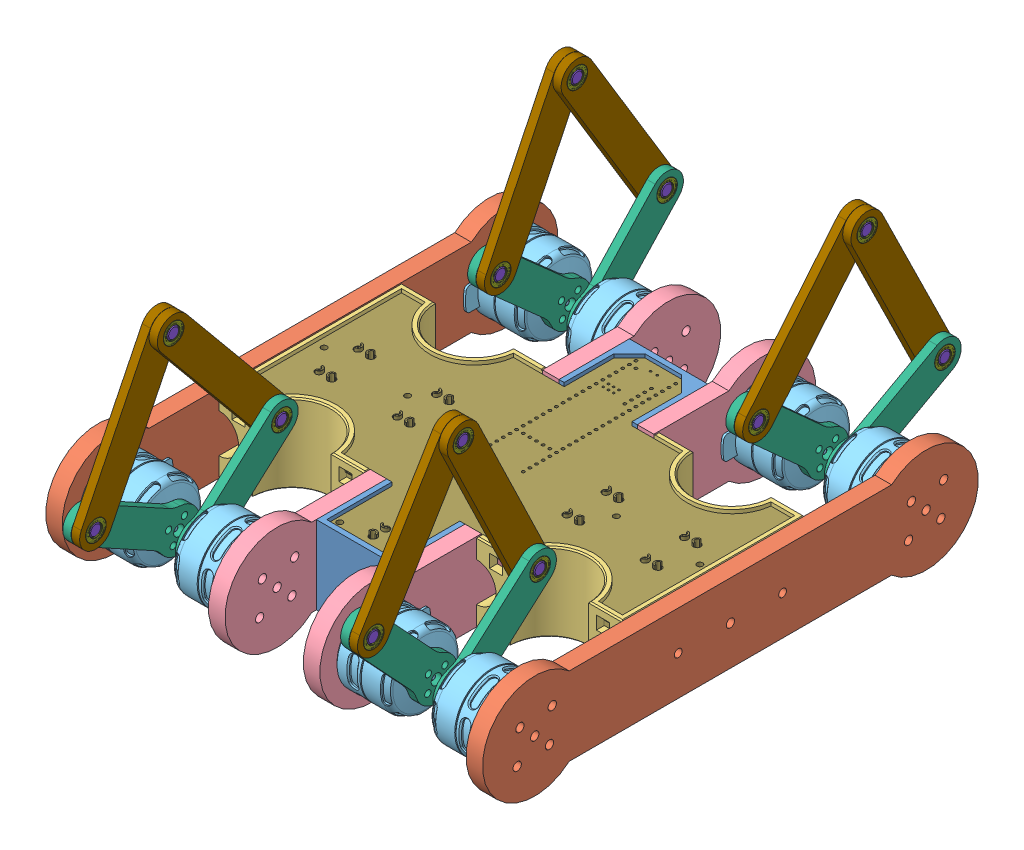
SolidWorks assembly microtaur, configuration Default. Lengths in mm.
Overall size (332.02 158.65 258.86).
76 component instances, 12 part files, 12 mates.
Components (placement in the parent):
- main_body_v2-1: main_body_v2 [Default] at origin size (30 30 120)
- leg_module-1: leg_module [Default] at (-54.7252 108.5431 -150.2745) x (-0.913523 -0.224854 0.338993) z (0.237532 -0.971371 -0.004207) size (136.16 215.13 114.83)
  - Beam_1-1: Beam_1 [Default] at (92.6439 -126.731 84.8587) x (-0.338993 0.940779 0.004207) z (0.913523 0.330234 -0.237532) size (190 40 6.35)
  - beam_spacer-1: beam_spacer [Default] at (92.6439 -126.731 84.8587) x (-0.338993 0.940779 0.004207) z (0.224854 0.076678 0.971371) size (70 56 30)
  - Beam_2-1: Beam_2 [Default] at (41.4866 -145.2241 98.1605) x (-0.338993 0.940779 0.004207) z (-0.913523 -0.330234 0.237532) size (190 40 6.35)
  - IQ2306 Distributable-8: IQ2306 Distributable [Default] at (16.0621 -74.6656 98.476) x (0.338993 -0.940779 -0.004207) z (0.913523 0.330234 -0.237532) size (33.2 28.4 23.5)
  - IQ2306 Distributable-11: IQ2306 Distributable [Default] at (118.0684 -197.2894 84.5431) x (-0.338993 0.940779 0.004207) z (-0.913523 -0.330234 0.237532) size (33.2 28.4 23.5)
  - IQ2306 Distributable-10: IQ2306 Distributable [Default] at (66.9111 -215.7825 97.8449) x (-0.338993 0.940779 0.004207) z (0.913523 0.330234 -0.237532) size (33.2 28.4 23.5)
  - IQ2306 Distributable-9: IQ2306 Distributable [Default] at (67.2194 -56.1725 85.1742) x (0.338993 -0.940779 -0.004207) z (-0.913523 -0.330234 0.237532) size (33.2 28.4 23.5)
  - Leg-1: Leg [Default] at (1.4498 6.4553 14.5504) x (0.999645 -0.014909 -0.022094) z (0.021162 -0.059998 0.997974) size (38.75 76.68 93.56) (flexible)
    - LegLink1-1: LegLink1 [Default] at (89.4523 -207.634 91.9838) x (0.397415 -0.599899 0.694393) z (0.086818 -0.728743 -0.679262) size (54.25 3.17 16)
    - 3759T53_Precision Stainless Steel Ball Bearing-1: 3759T53_Precision Stainless Steel Ball Bearing [3759T53] at (72.1055 -184.1623 64.5851) x (0.325654 -0.243773 0.913523) z (-0.913523 -0.330234 0.237532) size (7.94 7.94 3.17)
    - 98381A501_Dowel Pin-1: 98381A501_Dowel Pin [98381A501] at (73.5557 -183.638 64.2081) x (0.913523 0.330234 -0.237532) z (0.237532 0.040993 0.970514) size (6.35 4.76 4.76)
    - 98381A501_Dowel Pin-2: 98381A501_Dowel Pin [98381A501] at (104.0124 -240.8367 73.8233) x (-0.913523 -0.330234 0.237532) z (-0.212196 0.885033 0.414354) size (6.35 4.76 4.76)
    - LegLink1-2: LegLink1 [Default] at (95.5272 -205.438 90.4042) x (-0.212129 0.88497 0.414524) z (-0.347098 0.32829 -0.878492) size (54.25 3.17 16)
    - 3759T53_Precision Stainless Steel Ball Bearing-2: 3759T53_Precision Stainless Steel Ball Bearing [3759T53] at (105.4626 -240.3125 73.4462) x (-0.306532 0.942702 0.131724) z (0.913523 0.330234 -0.237532) size (7.94 7.94 3.17)
    - LegLink2-1: LegLink2 [Default] at (93.8016 -232.2122 46.965) x (-0.337315 0.288586 -0.896067) z (-0.227364 0.898701 0.375023) size (72.5 3.17 12.5)
    - 3759T53_Precision Stainless Steel Ball Bearing-3: 3759T53_Precision Stainless Steel Ball Bearing [3759T53] at (102.4708 -241.394 74.2241) x (0.325654 -0.243773 0.913523) z (-0.913523 -0.330234 0.237532) size (7.94 7.94 3.17)
    - LegLink2-2: LegLink2 [Default] at (75.7185 -204.6448 42.8997) x (0.069047 -0.701327 -0.709488) z (0.400884 -0.631732 0.66348) size (72.5 3.17 12.5)
    - 3759T53_Precision Stainless Steel Ball Bearing-4: 3759T53_Precision Stainless Steel Ball Bearing [3759T53] at (75.0973 -183.0808 63.8072) x (-0.306532 0.942702 0.131724) z (0.913523 0.330234 -0.237532) size (7.94 7.94 3.17)
    - 3759T53_Precision Stainless Steel Ball Bearing-5: 3759T53_Precision Stainless Steel Ball Bearing [3759T53] at (79.2401 -225.1604 21.238) x (-0.306532 0.942702 0.131724) z (0.913523 0.330234 -0.237532) size (7.94 7.94 3.17)
    - 3759T53_Precision Stainless Steel Ball Bearing-7: 3759T53_Precision Stainless Steel Ball Bearing [3759T53] at (82.2319 -224.0789 20.46) x (0.386893 -0.524966 0.758106) z (-0.913523 -0.330234 0.237532) size (7.94 7.94 3.17)
    - 98381A501_Dowel Pin-3: 98381A501_Dowel Pin [98381A501] at (80.6904 -224.6361 20.8609) x (0.913523 0.330234 -0.237532) z (0.3504 -0.935414 0.04712) size (6.35 4.76 4.76)
  - Leg-2: Leg [Default] at (-52.6711 118.3451 -38.0356) x (0.997195 0.048662 0.056866) z (-0.064222 0.166152 0.984007) size (38.75 76.68 93.56) (flexible)
    - LegLink1-1: LegLink1 [Default] at (89.4523 -207.634 91.9838) x (0.406276 -0.711409 0.573443) z (0.020389 -0.620357 -0.784054) size (54.25 3.17 16)
    - 3759T53_Precision Stainless Steel Ball Bearing-1: 3759T53_Precision Stainless Steel Ball Bearing [3759T53] at (71.7511 -179.7019 69.4231) x (0.325654 -0.243773 0.913523) z (-0.913523 -0.330234 0.237532) size (7.94 7.94 3.17)
    - 98381A501_Dowel Pin-1: 98381A501_Dowel Pin [98381A501] at (73.2013 -179.1777 69.0461) x (0.913523 0.330234 -0.237532) z (0.237532 0.040993 0.970514) size (6.35 4.76 4.76)
    - 98381A501_Dowel Pin-2: 98381A501_Dowel Pin [98381A501] at (96.7524 -230.9621 59.6306) x (-0.913523 -0.330234 0.237532) z (-0.212196 0.885033 0.414354) size (6.35 4.76 4.76)
    - LegLink1-2: LegLink1 [Default] at (95.5272 -205.438 90.4042) x (-0.03063 0.638103 0.769341) z (-0.405633 0.695535 -0.593037) size (54.25 3.17 16)
    - 3759T53_Precision Stainless Steel Ball Bearing-2: 3759T53_Precision Stainless Steel Ball Bearing [3759T53] at (98.2026 -230.4378 59.2535) x (-0.306532 0.942702 0.131724) z (0.913523 0.330234 -0.237532) size (7.94 7.94 3.17)
    - LegLink2-1: LegLink2 [Default] at (85.1997 -216.116 36.261) x (-0.382047 0.495972 -0.779777) z (-0.1397 0.803092 0.579247) size (72.5 3.17 12.5)
    - 3759T53_Precision Stainless Steel Ball Bearing-3: 3759T53_Precision Stainless Steel Ball Bearing [3759T53] at (95.2109 -231.5194 60.0314) x (0.325654 -0.243773 0.913523) z (-0.913523 -0.330234 0.237532) size (7.94 7.94 3.17)
    - LegLink2-2: LegLink2 [Default] at (70.5693 -191.2557 41.711) x (-0.090776 -0.403703 -0.910375) z (0.396529 -0.853211 0.338814) size (72.5 3.17 12.5)
    - 3759T53_Precision Stainless Steel Ball Bearing-4: 3759T53_Precision Stainless Steel Ball Bearing [3759T53] at (74.7428 -178.6204 68.6452) x (-0.306532 0.942702 0.131724) z (0.913523 0.330234 -0.237532) size (7.94 7.94 3.17)
    - 3759T53_Precision Stainless Steel Ball Bearing-5: 3759T53_Precision Stainless Steel Ball Bearing [3759T53] at (69.2963 -202.8426 14.0227) x (-0.306532 0.942702 0.131724) z (0.913523 0.330234 -0.237532) size (7.94 7.94 3.17)
    - 3759T53_Precision Stainless Steel Ball Bearing-7: 3759T53_Precision Stainless Steel Ball Bearing [3759T53] at (72.288 -201.7611 13.2448) x (0.386893 -0.524966 0.758106) z (-0.913523 -0.330234 0.237532) size (7.94 7.94 3.17)
    - 98381A501_Dowel Pin-3: 98381A501_Dowel Pin [98381A501] at (70.7465 -202.3183 13.6456) x (0.913523 0.330234 -0.237532) z (0.3504 -0.935414 0.04712) size (6.35 4.76 4.76)
- leg_module-2: leg_module [Default] at (54.7252 108.5431 150.2745) x (0.913523 -0.224854 -0.338993) z (-0.237532 -0.971371 0.004207) size (136.16 215.13 114.83)
  - Beam_1-1: Beam_1 [Default] at (92.6439 -126.731 84.8587) x (-0.338993 0.940779 0.004207) z (0.913523 0.330234 -0.237532) size (190 40 6.35)
  - beam_spacer-1: beam_spacer [Default] at (92.6439 -126.731 84.8587) x (-0.338993 0.940779 0.004207) z (0.224854 0.076678 0.971371) size (70 56 30)
  - Beam_2-1: Beam_2 [Default] at (41.4866 -145.2241 98.1605) x (-0.338993 0.940779 0.004207) z (-0.913523 -0.330234 0.237532) size (190 40 6.35)
  - IQ2306 Distributable-8: IQ2306 Distributable [Default] at (16.0621 -74.6656 98.476) x (0.338993 -0.940779 -0.004207) z (0.913523 0.330234 -0.237532) size (33.2 28.4 23.5)
  - IQ2306 Distributable-11: IQ2306 Distributable [Default] at (118.0684 -197.2894 84.5431) x (-0.338993 0.940779 0.004207) z (-0.913523 -0.330234 0.237532) size (33.2 28.4 23.5)
  - IQ2306 Distributable-10: IQ2306 Distributable [Default] at (66.9111 -215.7825 97.8449) x (-0.338993 0.940779 0.004207) z (0.913523 0.330234 -0.237532) size (33.2 28.4 23.5)
  - IQ2306 Distributable-9: IQ2306 Distributable [Default] at (67.2194 -56.1725 85.1742) x (0.338993 -0.940779 -0.004207) z (-0.913523 -0.330234 0.237532) size (33.2 28.4 23.5)
  - Leg-1: Leg [Default] at (1.4498 6.4553 14.5504) x (0.999645 -0.014909 -0.022094) z (0.021162 -0.059998 0.997974) size (38.75 76.68 93.56) (flexible)
    - LegLink1-1: LegLink1 [Default] at (89.4523 -207.634 91.9838) x (0.397415 -0.599899 0.694393) z (0.086818 -0.728743 -0.679262) size (54.25 3.17 16)
    - 3759T53_Precision Stainless Steel Ball Bearing-1: 3759T53_Precision Stainless Steel Ball Bearing [3759T53] at (72.1055 -184.1623 64.5851) x (0.325654 -0.243773 0.913523) z (-0.913523 -0.330234 0.237532) size (7.94 7.94 3.17)
    - 98381A501_Dowel Pin-1: 98381A501_Dowel Pin [98381A501] at (73.5557 -183.638 64.2081) x (0.913523 0.330234 -0.237532) z (0.237532 0.040993 0.970514) size (6.35 4.76 4.76)
    - 98381A501_Dowel Pin-2: 98381A501_Dowel Pin [98381A501] at (104.0124 -240.8367 73.8233) x (-0.913523 -0.330234 0.237532) z (-0.212196 0.885033 0.414354) size (6.35 4.76 4.76)
    - LegLink1-2: LegLink1 [Default] at (95.5272 -205.438 90.4042) x (-0.212129 0.88497 0.414524) z (-0.347098 0.32829 -0.878492) size (54.25 3.17 16)
    - 3759T53_Precision Stainless Steel Ball Bearing-2: 3759T53_Precision Stainless Steel Ball Bearing [3759T53] at (105.4626 -240.3125 73.4462) x (-0.306532 0.942702 0.131724) z (0.913523 0.330234 -0.237532) size (7.94 7.94 3.17)
    - LegLink2-1: LegLink2 [Default] at (93.8016 -232.2122 46.965) x (-0.337315 0.288586 -0.896067) z (-0.227364 0.898701 0.375023) size (72.5 3.17 12.5)
    - 3759T53_Precision Stainless Steel Ball Bearing-3: 3759T53_Precision Stainless Steel Ball Bearing [3759T53] at (102.4708 -241.394 74.2241) x (0.325654 -0.243773 0.913523) z (-0.913523 -0.330234 0.237532) size (7.94 7.94 3.17)
    - LegLink2-2: LegLink2 [Default] at (75.7185 -204.6448 42.8997) x (0.069047 -0.701327 -0.709488) z (0.400884 -0.631732 0.66348) size (72.5 3.17 12.5)
    - 3759T53_Precision Stainless Steel Ball Bearing-4: 3759T53_Precision Stainless Steel Ball Bearing [3759T53] at (75.0973 -183.0808 63.8072) x (-0.306532 0.942702 0.131724) z (0.913523 0.330234 -0.237532) size (7.94 7.94 3.17)
    - 3759T53_Precision Stainless Steel Ball Bearing-5: 3759T53_Precision Stainless Steel Ball Bearing [3759T53] at (79.2401 -225.1604 21.238) x (-0.306532 0.942702 0.131724) z (0.913523 0.330234 -0.237532) size (7.94 7.94 3.17)
    - 3759T53_Precision Stainless Steel Ball Bearing-7: 3759T53_Precision Stainless Steel Ball Bearing [3759T53] at (82.2319 -224.0789 20.46) x (0.386893 -0.524966 0.758106) z (-0.913523 -0.330234 0.237532) size (7.94 7.94 3.17)
    - 98381A501_Dowel Pin-3: 98381A501_Dowel Pin [98381A501] at (80.6904 -224.6361 20.8609) x (0.913523 0.330234 -0.237532) z (0.3504 -0.935414 0.04712) size (6.35 4.76 4.76)
  - Leg-2: Leg [Default] at (-52.6711 118.3451 -38.0356) x (0.997195 0.048662 0.056866) z (-0.064222 0.166152 0.984007) size (38.75 76.68 93.56) (flexible)
    - LegLink1-1: LegLink1 [Default] at (89.4523 -207.634 91.9838) x (0.406276 -0.711409 0.573443) z (0.020389 -0.620357 -0.784054) size (54.25 3.17 16)
    - 3759T53_Precision Stainless Steel Ball Bearing-1: 3759T53_Precision Stainless Steel Ball Bearing [3759T53] at (71.7511 -179.7019 69.4231) x (0.325654 -0.243773 0.913523) z (-0.913523 -0.330234 0.237532) size (7.94 7.94 3.17)
    - 98381A501_Dowel Pin-1: 98381A501_Dowel Pin [98381A501] at (73.2013 -179.1777 69.0461) x (0.913523 0.330234 -0.237532) z (0.237532 0.040993 0.970514) size (6.35 4.76 4.76)
    - 98381A501_Dowel Pin-2: 98381A501_Dowel Pin [98381A501] at (96.7524 -230.9621 59.6306) x (-0.913523 -0.330234 0.237532) z (-0.212196 0.885033 0.414354) size (6.35 4.76 4.76)
    - LegLink1-2: LegLink1 [Default] at (95.5272 -205.438 90.4042) x (-0.03063 0.638103 0.769341) z (-0.405633 0.695535 -0.593037) size (54.25 3.17 16)
    - 3759T53_Precision Stainless Steel Ball Bearing-2: 3759T53_Precision Stainless Steel Ball Bearing [3759T53] at (98.2026 -230.4378 59.2535) x (-0.306532 0.942702 0.131724) z (0.913523 0.330234 -0.237532) size (7.94 7.94 3.17)
    - LegLink2-1: LegLink2 [Default] at (85.1997 -216.116 36.261) x (-0.382047 0.495972 -0.779777) z (-0.1397 0.803092 0.579247) size (72.5 3.17 12.5)
    - 3759T53_Precision Stainless Steel Ball Bearing-3: 3759T53_Precision Stainless Steel Ball Bearing [3759T53] at (95.2109 -231.5194 60.0314) x (0.325654 -0.243773 0.913523) z (-0.913523 -0.330234 0.237532) size (7.94 7.94 3.17)
    - LegLink2-2: LegLink2 [Default] at (70.5693 -191.2557 41.711) x (-0.090776 -0.403703 -0.910375) z (0.396529 -0.853211 0.338814) size (72.5 3.17 12.5)
    - 3759T53_Precision Stainless Steel Ball Bearing-4: 3759T53_Precision Stainless Steel Ball Bearing [3759T53] at (74.7428 -178.6204 68.6452) x (-0.306532 0.942702 0.131724) z (0.913523 0.330234 -0.237532) size (7.94 7.94 3.17)
    - 3759T53_Precision Stainless Steel Ball Bearing-5: 3759T53_Precision Stainless Steel Ball Bearing [3759T53] at (69.2963 -202.8426 14.0227) x (-0.306532 0.942702 0.131724) z (0.913523 0.330234 -0.237532) size (7.94 7.94 3.17)
    - 3759T53_Precision Stainless Steel Ball Bearing-7: 3759T53_Precision Stainless Steel Ball Bearing [3759T53] at (72.288 -201.7611 13.2448) x (0.386893 -0.524966 0.758106) z (-0.913523 -0.330234 0.237532) size (7.94 7.94 3.17)
    - 98381A501_Dowel Pin-3: 98381A501_Dowel Pin [98381A501] at (70.7465 -202.3183 13.6456) x (0.913523 0.330234 -0.237532) z (0.3504 -0.935414 0.04712) size (6.35 4.76 4.76)
- battery-1: battery [Default] at (0.7274 -9.1118 -0.782) size (24 28 52)
- BNO055 breakout-1: BNO055 breakout [Default] at (0 14.1 -42.25) x (0 0 1) z (1 0 0) size (26.67 3.2 20.32)
- microtaur-teensy41-1: microtaur-teensy41 [Default] at (0 28.6 0) x (-1 0 0) z (0 -1 0) size (150.7 116.14 14.32)
Mates (geometry in assembly coordinates):
- Coincident14: coincident anti-aligned: plane of leg_module-1/Beam_1-1 through (-77.35 15 0) normal (0 0 -1)
- Coincident15: coincident anti-aligned: plane of main_body_v2-1 through (-15 30 60) normal (-1 0 0); plane of leg_module-1/Beam_2-1 through (-15 15 75) normal (1 0 0)
- Coincident17: coincident anti-aligned: plane of main_body_v2-1 through (15 30 60) normal (1 0 0); plane of leg_module-2/Beam_2-1 through (15 15 -75) normal (-1 0 0)
- Coincident19: coincident aligned: plane of leg_module-2/Beam_1-1 through (77.35 15 0) normal (0 0 1)
- Coincident23: coincident anti-aligned: plane of main_body_v2-1 through (-7.62 12.5 -31.455) normal (0 1 0); plane of BNO055 breakout-1 through (0 12.5 -42.25) normal (0 -1 0)
- Concentric3: concentric anti-aligned: cylinder of main_body_v2-1 through (-7.62 12.5 -53.045) axis (0 -1 0) radius 2.5; cylinder of BNO055 breakout-1 through (-7.62 12.5 -53.045) axis (0 1 0) radius 1.7078
- Concentric4: concentric anti-aligned: cylinder of main_body_v2-1 through (7.62 12.5 -53.045) axis (0 -1 0) radius 2.5; cylinder of BNO055 breakout-1 through (7.62 12.5 -53.045) axis (0 1 0) radius 1.7078
- Coincident24: coincident aligned: plane of main_body_v2-1 through (0 27 0) normal (0 1 0); plane of leg_module-2/Beam_2-1 through (11.35 27 -33) normal (0 1 0)
- Coincident25: coincident aligned: plane of main_body_v2-1 through (0 27 0) normal (0 1 0); plane of leg_module-1/Beam_2-1 through (-11.35 27 33) normal (0 1 0)
- Coincident26: coincident anti-aligned: plane of leg_module-2/beam_spacer-1 through (49.35 27 -35) normal (0 1 0); plane of microtaur-teensy41-1 through (0 27 0) normal (0 -1 0)
- Concentric5: concentric anti-aligned: cylinder of main_body_v2-1 through (11 27 55) axis (0 1 0) radius 1.25; cylinder of microtaur-teensy41-1 through (11 29.4 55) axis (0 -1 0) radius 1.1
- Concentric6: concentric anti-aligned: cylinder of main_body_v2-1 through (-11 27 55) axis (0 1 0) radius 1.25; cylinder of microtaur-teensy41-1 through (-11 29.4 55) axis (0 -1 0) radius 1.1
